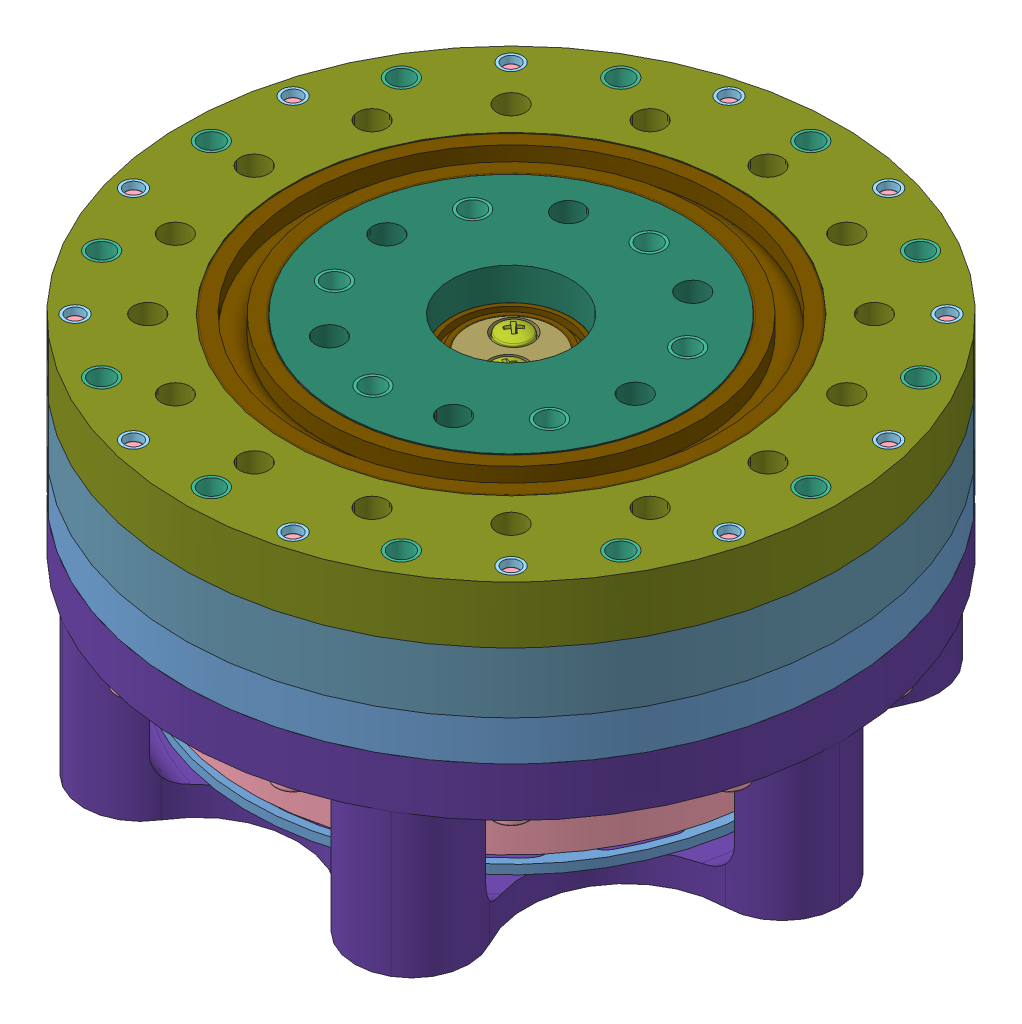
SolidWorks assembly Cycloidal, configuration Default. Lengths in mm. (continued)
Components (placement in the parent): (continued)
- foc-motor-controller.step-1: foc-motor-controller.step [Default] at (47.267 33.6573 89.1587) x (0.707107 0 0.707107) z (0 -1 0) size (57.23 50 8.13) (continued)
  - R_0603_1608Metric.step-6: R_0603_1608Metric.step [Default] at (10.9 4.1 1.595) size (1.6 0.8 0.45)
  - C_1206_3216Metric.step-2: C_1206_3216Metric.step [Default] at (6.3 11 1.595) x (0 1 0) z (0 0 1) size (3.2 1.6 1.6)
  - XT30PW_2_2_-M.G.B.step-1: XT30PW_2_2_-M.G.B.step [Default] at (-20.5 9.5 1.595) x (0 -1 0) z (-1 0 0) size (15.5 7.1 12.53)
  - R_0603_1608Metric.step-7: R_0603_1608Metric.step [Default] at (0.3 -11.1 1.595) size (1.6 0.8 0.45)
  - C_0603_1608Metric.step-6: C_0603_1608Metric.step [Default] at (19 -0.4 1.595) x (-0.707107 -0.707107 0) z (0 0 1) size (1.6 0.8 0.8)
  - C_1206_3216Metric.step-3: C_1206_3216Metric.step [Default] at (13.3 11 1.595) x (0 1 0) z (0 0 1) size (3.2 1.6 1.6)
  - R_0603_1608Metric.step-8: R_0603_1608Metric.step [Default] at (10.2 -7.375 1.595) x (0 -1 0) z (0 0 1) size (1.6 0.8 0.45)
  - JST_GH_SM08B-GHS-TB_1x08-1MP_P1.25mm_Horizontal.step-1: JST_GH_SM08B-GHS-TB_1x08-1MP_P1.25mm_Horizontal.step [Default] at (10 -22 1.595) size (13.25 4.95 4.25)
  - C_1206_3216Metric.step-4: C_1206_3216Metric.step [Default] at (-12.3 11 1.595) x (0 1 0) z (0 0 1) size (3.2 1.6 1.6)
  - JST_GH_SM06B-GHS-TB_1x06-1MP_P1.25mm_Horizontal.step-1: JST_GH_SM06B-GHS-TB_1x06-1MP_P1.25mm_Horizontal.step [Default] at (-4.3 -22 1.595) size (10.75 4.95 4.25)
  - C_0603_1608Metric.step-7: C_0603_1608Metric.step [Default] at (7.3 -4.5 1.595) x (-1 0 0) z (0 0 1) size (1.6 0.8 0.8)
  - R_0603_1608Metric.step-9: R_0603_1608Metric.step [Default] at (18.1 -3.86 1.595) x (-1 0 0) z (0 0 1) size (1.6 0.8 0.45)
  - C_1206_3216Metric.step-5: C_1206_3216Metric.step [Default] at (22.6794 -1.2206 1.595) x (0.707107 -0.707107 0) z (0 0 1) size (3.2 1.6 1.6)
  - R_Array_Convex_4x0402.step-1: R_Array_Convex_4x0402.step [Default] at (6.8 -2.5 1.595) size (1 2 0.35)
  - R_0603_1608Metric.step-10: R_0603_1608Metric.step [Default] at (7.7 -16.8 1.595) x (0 -1 0) z (0 0 1) size (1.6 0.8 0.45)
  - C_1206_3216Metric.step-6: C_1206_3216Metric.step [Default] at (8.7 11 1.595) x (0 1 0) z (0 0 1) size (3.2 1.6 1.6)
  - C_0603_1608Metric.step-8: C_0603_1608Metric.step [Default] at (16.1 -11.3 1.595) x (0 1 0) z (0 0 1) size (1.6 0.8 0.8)
  - SOT-23-5.step-1: SOT-23-5.step [Default] at (-3.1 -16.6 1.595) x (-1 0 0) z (0 0 1) size (2.8 2.9 1.55)
  - C_0603_1608Metric.step-9: C_0603_1608Metric.step [Default] at (17.8 -13.6 1.595) size (1.6 0.8 0.8)
  - R_0603_1608Metric.step-11: R_0603_1608Metric.step [Default] at (-11.5 -20.3875 1.595) x (0 -1 0) z (0 0 1) size (1.6 0.8 0.45)
  - C_0603_1608Metric.step-10: C_0603_1608Metric.step [Default] at (-12.4 2.3 1.595) x (0 1 0) z (0 0 1) size (1.6 0.8 0.8)
  - C_1206_3216Metric.step-7: C_1206_3216Metric.step [Default] at (18 11 1.595) x (0 1 0) z (0 0 1) size (3.2 1.6 1.6)
  - R_0603_1608Metric.step-12: R_0603_1608Metric.step [Default] at (-10.8105 -14.9971 1.595) x (-1 0 0) z (0 0 1) size (1.6 0.8 0.45)
  - C_0603_1608Metric.step-11: C_0603_1608Metric.step [Default] at (-13.8 -9.4 1.595) x (-1 0 0) z (0 0 1) size (1.6 0.8 0.8)
  - R_0603_1608Metric.step-13: R_0603_1608Metric.step [Default] at (-23.15 -14.5 1.595) x (-1 0 0) z (0 0 1) size (1.6 0.8 0.45)
  - C_0603_1608Metric.step-12: C_0603_1608Metric.step [Default] at (1.1 -0.2 1.595) x (0 1 0) z (0 0 1) size (1.6 0.8 0.8)
  - D_0805_2012Metric.step-1: D_0805_2012Metric.step [Default] at (22.9 -9.6 1.595) x (0 1 0) z (0 0 1) size (2 1.27 0.8)
  - C_0603_1608Metric.step-13: C_0603_1608Metric.step [Default] at (-7.8 3.775 1.595) x (0 -1 0) z (0 0 1) size (1.6 0.8 0.8)
  - R_0603_1608Metric.step-14: R_0603_1608Metric.step [Default] at (-6.4 -12.825 1.595) x (0 1 0) z (0 0 1) size (1.6 0.8 0.45)
  - L_0603_1608Metric.step-1: L_0603_1608Metric.step [Default] at (-10.1 3 1.595) size (1.6 0.8 0.8)
  - C_0603_1608Metric.step-14: C_0603_1608Metric.step [Default] at (17.9 0.7 1.595) x (-0.707107 -0.707107 0) z (0 0 1) size (1.6 0.8 0.8)
  - HVSSOP-10.step-1: HVSSOP-10.step [Default] at (18.6 -9.6 1.595) x (0 -1 0) z (-1 0 0) size (4.9 1.1 3)
  - C_0603_1608Metric.step-15: C_0603_1608Metric.step [Default] at (7.9 4.1 1.595) x (-1 0 0) z (0 0 1) size (1.6 0.8 0.8)
  - C_0603_1608Metric.step-16: C_0603_1608Metric.step [Default] at (21.1 -9.6 1.595) x (0 -1 0) z (0 0 1) size (1.6 0.8 0.8)
  - R_0603_1608Metric.step-15: R_0603_1608Metric.step [Default] at (-10.8105 -11.9971 1.595) x (-1 0 0) z (0 0 1) size (1.6 0.8 0.45)
  - R_0603_1608Metric.step-16: R_0603_1608Metric.step [Default] at (-18.2 -17.4 1.595) size (1.6 0.8 0.45)
  - C_1206_3216Metric.step-8: C_1206_3216Metric.step [Default] at (-3 11 1.595) x (0 1 0) z (0 0 1) size (3.2 1.6 1.6)
  - R_0603_1608Metric.step-17: R_0603_1608Metric.step [Default] at (-16.9 -20.4 1.595) x (0 -1 0) z (0 0 1) size (1.6 0.8 0.45)
  - R_0603_1608Metric.step-18: R_0603_1608Metric.step [Default] at (-13.3 -20.3875 1.595) x (0 -1 0) z (0 0 1) size (1.6 0.8 0.45)
  - R_0603_1608Metric.step-19: R_0603_1608Metric.step [Default] at (-15.1 -20.3875 1.595) x (0 -1 0) z (0 0 1) size (1.6 0.8 0.45)
  - C_0603_1608Metric.step-17: C_0603_1608Metric.step [Default] at (15.5 -14.4 1.595) x (0 -1 0) z (0 0 1) size (1.6 0.8 0.8)
  - LED_0603_1608Metric.step-1: LED_0603_1608Metric.step [Default] at (-11.5 -23.3875 1.595) x (0 1 0) z (0 0 1) size (1.6 0.8 1.1)
  - C_0805_2012Metric.step-1: C_0805_2012Metric.step [Default] at (19.95 -17 1.595) size (2 1.25 1.25)
  - D_SMB.step-1: D_SMB.step [Default] at (-16.5 11.208 1.595) x (0 -1 0) z (0 0 1) size (5.3 3.55 2.15)
  - C_1206_3216Metric.step-9: C_1206_3216Metric.step [Default] at (-5.3 11 1.595) x (0 1 0) z (0 0 1) size (3.2 1.6 1.6)
  - XT30PW_2_2_-M.G.B.step-2: XT30PW_2_2_-M.G.B.step [Default] at (-20.5 -6.5 1.595) x (0 -1 0) z (-1 0 0) size (15.5 7.1 12.53)
  - C_1206_3216Metric.step-10: C_1206_3216Metric.step [Default] at (1.7 11 1.595) x (0 1 0) z (0 0 1) size (3.2 1.6 1.6)
  - C_1206_3216Metric.step-11: C_1206_3216Metric.step [Default] at (11 11 1.595) x (0 1 0) z (0 0 1) size (3.2 1.6 1.6)
  - C_0603_1608Metric.step-18: C_0603_1608Metric.step [Default] at (-6.3 3.775 1.595) x (0 -1 0) z (0 0 1) size (1.6 0.8 0.8)
  - C_0603_1608Metric.step-19: C_0603_1608Metric.step [Default] at (16.8686 1.7314 1.595) x (0.707107 0.707107 0) z (0 0 1) size (1.6 0.8 0.8)
  - C_0603_1608Metric.step-20: C_0603_1608Metric.step [Default] at (-15.0105 -11.1 1.595) size (1.6 0.8 0.8)
  - C_1206_3216Metric.step-12: C_1206_3216Metric.step [Default] at (-7.7 11 1.595) x (0 1 0) z (0 0 1) size (3.2 1.6 1.6)
  - C_0603_1608Metric.step-21: C_0603_1608Metric.step [Default] at (-18.2 -15.8 1.595) size (1.6 0.8 0.8)
  - C_0603_1608Metric.step-22: C_0603_1608Metric.step [Default] at (-2.1 -11.3 1.595) x (0 -1 0) z (0 0 1) size (1.6 0.8 0.8)
  - C_0603_1608Metric.step-23: C_0603_1608Metric.step [Default] at (-10.8105 -13.4971 1.595) size (1.6 0.8 0.8)
  - C_1206_3216Metric.step-13: C_1206_3216Metric.step [Default] at (4 11 1.595) x (0 1 0) z (0 0 1) size (3.2 1.6 1.6)
  - R_0603_1608Metric.step-20: R_0603_1608Metric.step [Default] at (16 -17.8 1.595) x (0 1 0) z (0 0 1) size (1.6 0.8 0.45)
  - Texas_S-PVSON-N8.step-1: Texas_S-PVSON-N8.step [Default] at (-14.4105 -13.7 1.595) x (-1 0 0) z (0 0 1) size (3 2.98 0.92)
  - C_1206_3216Metric.step-14: C_1206_3216Metric.step [Default] at (21 -2.9 1.595) x (0.707107 -0.707107 0) z (0 0 1) size (3.2 1.6 1.6)
  - C_0603_1608Metric.step-24: C_0603_1608Metric.step [Default] at (-5.9 -16.6 1.595) x (0 1 0) z (0 0 1) size (1.6 0.8 0.8)
  - C_0603_1608Metric.step-25: C_0603_1608Metric.step [Default] at (-3.1 -14.1 1.595) size (1.6 0.8 0.8)
  - R_0603_1608Metric.step-21: R_0603_1608Metric.step [Default] at (7.2 -7.375 1.595) x (0 -1 0) z (0 0 1) size (1.6 0.8 0.45)
  - C_1206_3216Metric.step-15: C_1206_3216Metric.step [Default] at (-0.7 11 1.595) x (0 1 0) z (0 0 1) size (3.2 1.6 1.6)
  - LQFP-64_10x10mm_P0.5mm.step-1: LQFP-64_10x10mm_P0.5mm.step [Default] at (-7 -4.5 1.595) x (-1 0 0) z (0 0 1) size (12 12 1.5)
  - C_0805_2012Metric.step-2: C_0805_2012Metric.step [Default] at (23.35 -17 1.595) x (-1 0 0) z (0 0 1) size (2 1.25 1.25)
  - C_0603_1608Metric.step-26: C_0603_1608Metric.step [Default] at (10.8 -16.8 1.595) x (0 -1 0) z (0 0 1) size (1.6 0.8 0.8)
  - R_0603_1608Metric.step-22: R_0603_1608Metric.step [Default] at (17.5 -17.8 1.595) x (0 -1 0) z (0 0 1) size (1.6 0.8 0.45)
  - C_1206_3216Metric.step-16: C_1206_3216Metric.step [Default] at (20.3 11 1.595) x (0 1 0) z (0 0 1) size (3.2 1.6 1.6)
  - R_0603_1608Metric.step-23: R_0603_1608Metric.step [Default] at (9.2 -16.8 1.595) x (0 -1 0) z (0 0 1) size (1.6 0.8 0.45)
  - C_1206_3216Metric.step-17: C_1206_3216Metric.step [Default] at (-10 11 1.595) x (0 1 0) z (0 0 1) size (3.2 1.6 1.6)
  - R_0603_1608Metric.step-24: R_0603_1608Metric.step [Default] at (17.8 -15.2 1.595) size (1.6 0.8 0.45)
  - C_1206_3216Metric.step-18: C_1206_3216Metric.step [Default] at (19.9 2.6 1.595) x (-0.707107 0.707107 0) z (0 0 1) size (3.2 1.6 1.6)
  - C_0603_1608Metric.step-27: C_0603_1608Metric.step [Default] at (13.4 -7.375 1.595) x (0 -1 0) z (0 0 1) size (1.6 0.8 0.8)
  - R_0603_1608Metric.step-25: R_0603_1608Metric.step [Default] at (8.7 -7.375 1.595) x (0 -1 0) z (0 0 1) size (1.6 0.8 0.45)
  - PQFN-8-EP_6x5mm_P1.27mm_Generic.step-1: PQFN-8-EP_6x5mm_P1.27mm_Generic.step [Default] at (4.9 14.4 -0.085) x (0 1 0) z (0 0 -1) size (6.15 5.15 1.09)
  - C_0805_2012Metric.step-3: C_0805_2012Metric.step [Default] at (-3 8.9 -0.085) x (0 1 0) z (0 0 -1) size (2 1.25 1.25)
  - C_0603_1608Metric.step-28: C_0603_1608Metric.step [Default] at (1.5 -4.3 -0.085) x (0 1 0) z (0 0 -1) size (1.6 0.8 0.8)
  - R_2512_6332Metric.step-1: R_2512_6332Metric.step [Default] at (2.1 8.6 -0.085) x (-1 0 0) z (0 0 -1) size (6.3 3.2 0.6)
  - C_0805_2012Metric.step-4: C_0805_2012Metric.step [Default] at (18.8 8.9 -0.085) x (0 1 0) z (0 0 -1) size (2 1.25 1.25)
  - C_0805_2012Metric.step-5: C_0805_2012Metric.step [Default] at (-5.2 8.901 -0.085) x (0 1 0) z (0 0 -1) size (2 1.25 1.25)
  - PQFN-8-EP_6x5mm_P1.27mm_Generic.step-2: PQFN-8-EP_6x5mm_P1.27mm_Generic.step [Default] at (16.9 14.6 -0.085) x (0 -1 0) z (0 0 -1) size (6.15 5.15 1.09)
  - PQFN-8-EP_6x5mm_P1.27mm_Generic.step-3: PQFN-8-EP_6x5mm_P1.27mm_Generic.step [Default] at (-1.1 14.6 -0.085) x (0 -1 0) z (0 0 -1) size (6.15 5.15 1.09)
  - R_0603_1608Metric.step-26: R_0603_1608Metric.step [Default] at (8.2 8.8 -0.085) x (0 1 0) z (0 0 -1) size (1.6 0.8 0.45)
  - R_2512_6332Metric.step-2: R_2512_6332Metric.step [Default] at (-10.3 8.601 -0.085) x (1 0 0) z (0 0 -1) size (6.3 3.2 0.6)
  - TSSOP-16_4.4x5mm_P0.65mm.step-1: TSSOP-16_4.4x5mm_P0.65mm.step [Default] at (0 0 -0.085) x (-1 0 0) z (0 0 -1) size (6.4 5 1.1)
  - C_0603_1608Metric.step-29: C_0603_1608Metric.step [Default] at (0 -4.25 -0.085) x (0 1 0) z (0 0 -1) size (1.6 0.8 0.8)
  - PQFN-8-EP_6x5mm_P1.27mm_Generic.step-4: PQFN-8-EP_6x5mm_P1.27mm_Generic.step [Default] at (10.9 14.4 -0.085) x (0 1 0) z (0 0 -1) size (6.15 5.15 1.09)
  - R_2512_6332Metric.step-3: R_2512_6332Metric.step [Default] at (13.7 8.6 -0.085) x (1 0 0) z (0 0 -1) size (6.3 3.2 0.6)
  - PQFN-8-EP_6x5mm_P1.27mm_Generic.step-5: PQFN-8-EP_6x5mm_P1.27mm_Generic.step [Default] at (-13.1 14.401 -0.085) x (0 1 0) z (0 0 -1) size (6.15 5.15 1.09)
  - C_0603_1608Metric.step-30: C_0603_1608Metric.step [Default] at (-1.5 -4.3 -0.085) x (0 -1 0) z (0 0 -1) size (1.6 0.8 0.8)
  - PQFN-8-EP_6x5mm_P1.27mm_Generic.step-6: PQFN-8-EP_6x5mm_P1.27mm_Generic.step [Default] at (-7.1 14.601 -0.085) x (0 -1 0) z (0 0 -1) size (6.15 5.15 1.09)
  - foc-motor-controller_PCB.step-1: foc-motor-controller_PCB.step [Default] at origin size (50 50 1.51)
- hex nut style 1 gradeab_iso-1: hex nut style 1 gradeab_iso [ISO - 4032 - M3 - W - N] at (47.267 33.6573 58.7531) x (1 0 0) z (0 -1 0) size (5.5 6.35 2.4)
Mates (geometry in assembly coordinates):
- Coincident1: coincident anti-aligned: plane of motor-X83008S.stp-1/outrunner.stp-1 through (20.8832 69.6573 111.3881) normal (0 1 0); plane of Base_Plate-1 through (47.267 69.6573 89.1587) normal (0 -1 0)
- Concentric1: concentric anti-aligned: line of motor-X83008S.stp-1/outrunner.stp-1 through (35.4134 64.1573 99.1458) axis (0 1 0); cylinder of Base_Plate-1 through (35.4134 76.6573 99.1458) axis (0 -1 0) radius 1.5
- Concentric2: concentric anti-aligned: cylinder of motor-X83008S.stp-1/shaft.stp-1 through (47.267 69.6573 89.1587) axis (0 1 0) radius 1.5; line of Base_Plate-1 through (47.267 76.6573 89.1587) axis (0 -1 0)
- Coincident2: coincident anti-aligned: plane of Base_Plate-1 through (47.267 76.6573 89.1587) normal (0 1 0); plane of Eccentric_Shaft-1/Eccentric_Shaft_bot-1 through (48.4141 76.6573 88.1922) normal (0 -1 0)
- Concentric75: concentric anti-aligned: cylinder of Output_Shaft-1 through (47.267 97.2573 89.1587) axis (0 -1 0) radius 30; cylinder of radial ball bearing_68_iso-39 through (47.267 71.6198 89.1587) axis (0 1 0) radius 30
- Concentric76: concentric anti-aligned: cylinder of Cover-1 through (47.267 97.2573 89.1587) axis (0 -1 0) radius 39; cylinder of radial ball bearing_68_iso-39 through (47.267 71.6198 89.1587) axis (0 1 0) radius 39
- Coincident104: coincident aligned: plane of Cover-1 through (47.267 97.2573 89.1587) normal (0 1 0); plane of radial ball bearing_68_iso-39 through (8.567 97.2573 89.1587) normal (0 1 0)
- Coincident105: coincident aligned: plane of Output_Shaft-1 through (47.267 97.2573 89.1587) normal (0 1 0); plane of Cover-1 through (47.267 97.2573 89.1587) normal (0 1 0)
- Concentric77: concentric aligned: cylinder of Ring_Pin_Housing-1 through (47.267 87.2573 89.1587) axis (0 -1 0) radius 57.5; cylinder of Motor_Cover-2 through (47.267 69.6573 89.1587) axis (0 -1 0) radius 57.5
- Concentric78: concentric anti-aligned: cylinder of Base_Plate-1 through (47.267 76.6573 89.1587) axis (0 -1 0) radius 20; cylinder of radial ball bearing_68_iso-40 through (47.267 52.3198 89.1587) axis (0 1 0) radius 20
- Concentric79: concentric aligned: cylinder of Ring_Pin_Housing-1 through (9.0832 87.2573 50.9749) axis (0 -1 0) radius 1.6; cylinder of Base_plate_2-1 through (9.0832 76.6573 50.9749) axis (0 -1 0) radius 1.75
- Concentric80: concentric aligned: cylinder of Ring_Pin_Housing-1 through (47.267 87.2573 89.1587) axis (0 -1 0) radius 57.5; cylinder of Base_plate_2-1 through (47.267 76.6573 89.1587) axis (0 -1 0) radius 57.5
- Coincident107: coincident anti-aligned: plane of Ring_Pin_Housing-1 through (47.267 76.6573 89.1587) normal (0 -1 0); plane of Base_plate_2-1 through (47.267 76.6573 89.1587) normal (0 1 0)
- Concentric83: concentric aligned: cylinder of Ring_Pin_Housing-1 through (9.0832 87.2573 50.9749) axis (0 -1 0) radius 1.6; cylinder of Cover-1 through (9.0832 97.2573 50.9749) axis (0 -1 0) radius 2
- Concentric84: concentric aligned: cylinder of Cover-1 through (15.4472 87.2573 57.3389) axis (0 1 0) radius 2.5; cylinder of m13_bearing-1/m6-1 through (15.4472 86.8573 57.3389) axis (0 1 0) radius 2
- Concentric85: concentric aligned: cylinder of Cover-1 through (47.267 87.2573 134.1587) axis (0 1 0) radius 2.5; cylinder of m13_bearing-11/m6-1 through (47.267 86.8573 134.1587) axis (0 1 0) radius 2
- Concentric86: concentric aligned: cylinder of Cover-1 through (64.4877 87.2573 130.7332) axis (0 1 0) radius 2.5; cylinder of m13_bearing-2/m6-1 through (64.4877 86.8573 130.7332) axis (0 1 0) radius 2
- Concentric87: concentric aligned: cylinder of Cover-1 through (79.0868 87.2573 120.9785) axis (0 1 0) radius 2.5; cylinder of m13_bearing-12/m6-1 through (79.0868 86.8573 120.9785) axis (0 1 0) radius 2
- Concentric88: concentric aligned: cylinder of Cover-1 through (88.8416 87.2573 106.3794) axis (0 1 0) radius 2.5; cylinder of m13_bearing-5/m6-1 through (88.8416 86.8573 106.3794) axis (0 1 0) radius 2
- Concentric89: concentric aligned: cylinder of Cover-1 through (92.267 87.2573 89.1587) axis (0 1 0) radius 2.5; cylinder of m13_bearing-4/m6-1 through (92.267 86.8573 89.1587) axis (0 1 0) radius 2
- Concentric90: concentric aligned: cylinder of Cover-1 through (30.0462 87.2573 47.5841) axis (0 1 0) radius 2.5; cylinder of m13_bearing-6/m6-1 through (30.0462 86.8573 47.5841) axis (0 1 0) radius 2
- Concentric91: concentric aligned: cylinder of Cover-1 through (47.267 87.2573 44.1587) axis (0 1 0) radius 2.5; cylinder of m13_bearing-3/m6-1 through (47.267 86.8573 44.1587) axis (0 1 0) radius 2
- Concentric92: concentric aligned: cylinder of Cover-1 through (64.4877 87.2573 47.5841) axis (0 1 0) radius 2.5; cylinder of m13_bearing-7/m6-1 through (64.4877 86.8573 47.5841) axis (0 1 0) radius 2
- Concentric93: concentric aligned: cylinder of Cover-1 through (79.0868 87.2573 57.3389) axis (0 1 0) radius 2.5; cylinder of m13_bearing-8/m6-1 through (79.0868 86.8573 57.3389) axis (0 1 0) radius 2
- Concentric94: concentric aligned: cylinder of Cover-1 through (88.8416 87.2573 71.9379) axis (0 1 0) radius 2.5; cylinder of m13_bearing-9/m6-1 through (88.8416 86.8573 71.9379) axis (0 1 0) radius 2
- Concentric96: concentric aligned: cylinder of Base_plate_2-1 through (47.267 76.6573 134.1587) axis (0 -1 0) radius 2.5; cylinder of socket button head screw_iso-2 through (47.267 67.4573 134.1587) axis (0 -1 0) radius 2
- Coincident121: coincident anti-aligned: plane of Base_plate_2-1 through (47.267 69.6573 89.1587) normal (0 -1 0); plane of socket button head screw_iso-2 through (45.8877 69.6573 132.7104) normal (0 1 0)
- Concentric971: concentric aligned: cylinder of Base_plate_2-1 through (15.4472 76.6573 57.3389) axis (0 -1 0) radius 2.5; cylinder of socket button head screw_iso-3 through (15.4472 67.4573 57.3389) axis (0 -1 0) radius 3.8
- Coincident1221: coincident anti-aligned: plane of Base_plate_2-1 through (47.267 69.6573 89.1587) normal (0 -1 0); plane of socket button head screw_iso-3 through (14.0679 69.6573 55.8906) normal (0 1 0)
- Concentric981: concentric aligned: cylinder of Base_plate_2-1 through (30.0462 76.6573 47.5841) axis (0 -1 0) radius 2.5; cylinder of socket button head screw_iso-4 through (30.0462 67.4573 47.5841) axis (0 -1 0) radius 3.8
- Coincident1231: coincident anti-aligned: plane of Base_plate_2-1 through (47.267 69.6573 89.1587) normal (0 -1 0); plane of socket button head screw_iso-4 through (28.6669 69.6573 46.1358) normal (0 1 0)
- Concentric991: concentric aligned: cylinder of Base_plate_2-1 through (47.267 76.6573 44.1587) axis (0 -1 0) radius 2.5; cylinder of socket button head screw_iso-5 through (47.267 67.4573 44.1587) axis (0 -1 0) radius 3.8
- Coincident1241: coincident anti-aligned: plane of Base_plate_2-1 through (47.267 69.6573 89.1587) normal (0 -1 0); plane of socket button head screw_iso-5 through (45.8877 69.6573 42.7104) normal (0 1 0)
- Concentric1001: concentric aligned: cylinder of Base_plate_2-1 through (64.4877 76.6573 47.5841) axis (0 -1 0) radius 2.5; cylinder of socket button head screw_iso-6 through (64.4877 67.4573 47.5841) axis (0 -1 0) radius 3.8
- Coincident1251: coincident anti-aligned: plane of Base_plate_2-1 through (47.267 69.6573 89.1587) normal (0 -1 0); plane of socket button head screw_iso-6 through (63.1085 69.6573 46.1358) normal (0 1 0)
- Concentric1021: concentric aligned: cylinder of Base_plate_2-1 through (88.8416 76.6573 71.9379) axis (0 -1 0) radius 2.5; cylinder of socket button head screw_iso-8 through (88.8416 67.4573 71.9379) axis (0 -1 0) radius 3.8
- Coincident1271: coincident anti-aligned: plane of Base_plate_2-1 through (47.267 69.6573 89.1587) normal (0 -1 0); plane of socket button head screw_iso-8 through (87.4623 69.6573 70.4896) normal (0 1 0)
- Concentric1031: concentric aligned: cylinder of Base_plate_2-1 through (92.267 76.6573 89.1587) axis (0 -1 0) radius 2.5; cylinder of socket button head screw_iso-9 through (92.267 67.4573 89.1587) axis (0 -1 0) radius 3.8
- Coincident1281: coincident anti-aligned: plane of Base_plate_2-1 through (47.267 69.6573 89.1587) normal (0 -1 0); plane of socket button head screw_iso-9 through (90.8877 69.6573 87.7104) normal (0 1 0)
- Concentric1041: concentric aligned: cylinder of Base_plate_2-1 through (88.8416 76.6573 106.3794) axis (0 -1 0) radius 2.5; cylinder of socket button head screw_iso-10 through (88.8416 67.4573 106.3794) axis (0 -1 0) radius 3.8
- Coincident1291: coincident anti-aligned: plane of Base_plate_2-1 through (47.267 69.6573 89.1587) normal (0 -1 0); plane of socket button head screw_iso-10 through (87.4623 69.6573 104.9311) normal (0 1 0)
- Concentric1051: concentric aligned: cylinder of Base_plate_2-1 through (79.0868 76.6573 120.9785) axis (0 -1 0) radius 2.5; cylinder of socket button head screw_iso-11 through (79.0868 67.4573 120.9785) axis (0 -1 0) radius 3.8
- Coincident1301: coincident anti-aligned: plane of Base_plate_2-1 through (47.267 69.6573 89.1587) normal (0 -1 0); plane of socket button head screw_iso-11 through (77.7075 69.6573 119.5302) normal (0 1 0)
- Coincident132: coincident anti-aligned: plane of Ring_Pin_Housing-1 through (47.267 87.2573 89.1587) normal (0 1 0); plane of Cover-1 through (47.267 87.2573 89.1587) normal (0 -1 0)
- Coincident133: coincident anti-aligned: plane of Motor_Cover-2 through (47.267 69.6573 89.1587) normal (0 1 0); plane of Base_plate_2-1 through (47.267 69.6573 89.1587) normal (0 -1 0)
- Concentric109: concentric anti-aligned: cylinder of Output_Shaft-1 through (24.2995 97.2573 87.9364) axis (0 -1 0) radius 2.5; cylinder of m13_bearing-14/m6-1 through (24.2995 86.4573 87.9364) axis (0 1 0) radius 2
- Concentric110: concentric anti-aligned: cylinder of Output_Shaft-1 through (36.8417 97.2573 68.6571) axis (0 -1 0) radius 2.5; cylinder of m13_bearing-13/m6-1 through (36.8417 86.4573 68.6571) axis (0 1 0) radius 2
- Concentric111: concentric anti-aligned: cylinder of Output_Shaft-1 through (59.8092 97.2573 69.8794) axis (0 -1 0) radius 2.5; cylinder of m13_bearing-16/m6-1 through (59.8092 86.4573 69.8794) axis (0 1 0) radius 2
- Concentric112: concentric anti-aligned: cylinder of Output_Shaft-1 through (70.2345 97.2573 90.3809) axis (0 -1 0) radius 2.5; cylinder of m13_bearing-18/m6-1 through (70.2345 86.4573 90.3809) axis (0 1 0) radius 2
- Concentric113: concentric anti-aligned: cylinder of Output_Shaft-1 through (57.6922 97.2573 109.6602) axis (0 -1 0) radius 2.5; cylinder of m13_bearing-17/m6-1 through (57.6922 86.4573 109.6602) axis (0 1 0) radius 2
- Concentric114: concentric anti-aligned: cylinder of Output_Shaft-1 through (34.7247 97.2573 108.438) axis (0 -1 0) radius 2.5; cylinder of m13_bearing-15/m6-1 through (34.7247 86.4573 108.438) axis (0 1 0) radius 2
- Coincident136: coincident aligned: plane of m13_bearing-13/m6-1 through (36.8417 92.4573 68.6571) normal (0 1 0); plane of m13_bearing-14/m6-1 through (24.2995 92.4573 87.9364) normal (0 1 0)
- Coincident137: coincident aligned: plane of m13_bearing-14/m6-1 through (24.2995 92.4573 87.9364) normal (0 1 0); plane of m13_bearing-16/m6-1 through (59.8092 92.4573 69.8794) normal (0 1 0)
- Coincident138: coincident aligned: plane of m13_bearing-14/m6-1 through (24.2995 92.4573 87.9364) normal (0 1 0); plane of m13_bearing-18/m6-1 through (70.2345 92.4573 90.3809) normal (0 1 0)
- Coincident139: coincident aligned: plane of m13_bearing-14/m6-1 through (24.2995 92.4573 87.9364) normal (0 1 0); plane of m13_bearing-17/m6-1 through (57.6922 92.4573 109.6602) normal (0 1 0)
- Coincident140: coincident aligned: plane of m13_bearing-14/m6-1 through (24.2995 92.4573 87.9364) normal (0 1 0); plane of m13_bearing-15/m6-1 through (34.7247 92.4573 108.438) normal (0 1 0)
- Concentric117: concentric anti-aligned: cylinder of Cover-1 through (9.0832 97.2573 127.3424) axis (0 -1 0) radius 2; cylinder of Motor_Cover-2 through (9.0832 59.6573 127.3424) axis (0 1 0) radius 1.75
- Concentric118: concentric anti-aligned: cylinder of Output_Shaft-1 through (36.8417 97.2573 68.6571) axis (0 -1 0) radius 2.5; cylinder of M4x6x5.5_brass_insert-1 through (36.8417 86.4573 68.6571) axis (0 1 0) radius 2
- Coincident144: coincident aligned: plane of Cover-1 through (47.267 97.2573 89.1587) normal (0 1 0); plane of M3x4x4.2_brass_insert-1 through (-2.9238 97.2573 74.8329) normal (0 1 0)
- Concentric1211: concentric aligned: cylinder of Cover-1 through (9.0832 97.2573 50.9749) axis (0 -1 0) radius 2; cylinder of M3x4x4.2_brass_insert-2 through (9.0832 92.3553 50.9749) axis (0 -1 0) radius 1.5
- Concentric1221: concentric aligned: cylinder of Cover-1 through (33.2908 97.2573 36.9987) axis (0 -1 0) radius 2; cylinder of M3x4x4.2_brass_insert-3 through (33.2908 92.3553 36.9987) axis (0 -1 0) radius 1.5
- Concentric1251: concentric aligned: cylinder of Cover-1 through (99.427 97.2573 75.1824) axis (0 -1 0) radius 2; cylinder of M3x4x4.2_brass_insert-6 through (99.427 92.3553 75.1824) axis (0 -1 0) radius 1.8
- Concentric1271: concentric anti-aligned: cylinder of Cover-1 through (85.4508 97.2573 127.3424) axis (0 -1 0) radius 2; cylinder of M3x4x4.2_brass_insert-8 through (85.4508 98.1594 127.3424) axis (0 1 0) radius 1.8
- Concentric1331: concentric aligned: cylinder of Cover-1 through (61.2432 97.2573 36.9987) axis (0 -1 0) radius 2; cylinder of M3x4x4.2_brass_insert-14 through (61.2432 92.3553 36.9987) axis (0 -1 0) radius 1.8
- Concentric1341: concentric anti-aligned: cylinder of Cover-1 through (85.4508 97.2573 50.9749) axis (0 -1 0) radius 2; cylinder of M3x4x4.2_brass_insert-15 through (85.4508 98.1594 50.9749) axis (0 1 0) radius 2
- Concentric1351: concentric aligned: cylinder of Cover-1 through (99.427 97.2573 103.1349) axis (0 -1 0) radius 2; cylinder of M3x4x4.2_brass_insert-16 through (99.427 92.3553 103.1349) axis (0 -1 0) radius 2
- Concentric1361: concentric aligned: cylinder of Cover-1 through (61.2432 97.2573 141.3187) axis (0 -1 0) radius 2; cylinder of M3x4x4.2_brass_insert-17 through (61.2432 92.3553 141.3187) axis (0 -1 0) radius 2
- Concentric1381: concentric aligned: cylinder of Cover-1 through (33.2908 97.2573 141.3187) axis (0 -1 0) radius 2; cylinder of M3x4x4.2_brass_insert-19 through (33.2908 92.3553 141.3187) axis (0 -1 0) radius 2
- Concentric1391: concentric aligned: cylinder of Cover-1 through (9.0832 97.2573 127.3424) axis (0 -1 0) radius 2; cylinder of M3x4x4.2_brass_insert-20 through (9.0832 92.3553 127.3424) axis (0 -1 0) radius 1.5
- Concentric1401: concentric aligned: cylinder of Cover-1 through (-4.893 97.2573 103.1349) axis (0 -1 0) radius 2; cylinder of M3x4x4.2_brass_insert-21 through (-4.893 92.3553 103.1349) axis (0 -1 0) radius 1.5
- Coincident205: coincident aligned: plane of M3x4x4.2_brass_insert-1 through (-2.9238 97.2573 74.8329) normal (0 1 0); plane of M3x4x4.2_brass_insert-2 through (8.0628 97.2573 49.8755) normal (0 1 0)
- Coincident206: coincident aligned: plane of M3x4x4.2_brass_insert-1 through (-2.9238 97.2573 74.8329) normal (0 1 0); plane of M3x4x4.2_brass_insert-3 through (32.5264 97.2573 35.708) normal (0 1 0)
- Coincident207: coincident aligned: plane of M3x4x4.2_brass_insert-1 through (-2.9238 97.2573 74.8329) normal (0 1 0); plane of M3x4x4.2_brass_insert-14 through (62.0075 97.2573 38.2893) normal (0 1 0)
- Coincident208: coincident aligned: plane of M3x4x4.2_brass_insert-1 through (-2.9238 97.2573 74.8329) normal (0 1 0); plane of M3x4x4.2_brass_insert-15 through (87.2451 97.2573 50.0916) normal (0 1 0)
- Coincident209: coincident aligned: plane of M3x4x4.2_brass_insert-1 through (-2.9238 97.2573 74.8329) normal (0 1 0); plane of M3x4x4.2_brass_insert-6 through (98.4066 97.2573 74.083) normal (0 1 0)
- Coincident210: coincident aligned: plane of M3x4x4.2_brass_insert-1 through (-2.9238 97.2573 74.8329) normal (0 1 0); plane of M3x4x4.2_brass_insert-16 through (98.4066 97.2573 102.0355) normal (0 1 0)
- Coincident211: coincident aligned: plane of M3x4x4.2_brass_insert-1 through (-2.9238 97.2573 74.8329) normal (0 1 0); plane of M3x4x4.2_brass_insert-8 through (83.51 97.2573 127.8255) normal (0 1 0)
- Coincident212: coincident aligned: plane of M3x4x4.2_brass_insert-1 through (-2.9238 97.2573 74.8329) normal (0 1 0); plane of M3x4x4.2_brass_insert-17 through (62.2636 97.2573 142.4181) normal (0 1 0)
- Coincident213: coincident aligned: plane of M3x4x4.2_brass_insert-1 through (-2.9238 97.2573 74.8329) normal (0 1 0); plane of M3x4x4.2_brass_insert-19 through (34.3112 97.2573 142.4181) normal (0 1 0)
- Coincident214: coincident aligned: plane of M3x4x4.2_brass_insert-1 through (-2.9238 97.2573 74.8329) normal (0 1 0); plane of M3x4x4.2_brass_insert-20 through (10.1036 97.2573 128.4419) normal (0 1 0)
- Coincident215: coincident aligned: plane of M3x4x4.2_brass_insert-1 through (-2.9238 97.2573 74.8329) normal (0 1 0); plane of M3x4x4.2_brass_insert-21 through (-3.8726 97.2573 104.2343) normal (0 1 0)
- Coincident1432: coincident aligned: plane of m13_bearing-13/m6-1 through (36.8417 92.4573 68.6571) normal (0 1 0); plane of M4x6x5.5_brass_insert-1 through (34.9772 92.4573 70.3224) normal (0 1 0)
- Concentric14021: concentric aligned: cylinder of Output_Shaft-1 through (70.2345 97.2573 90.3809) axis (0 -1 0) radius 2.5; cylinder of M4x6x5.5_brass_insert-4 through (70.2345 80.5133 90.3809) axis (0 -1 0) radius 2.5
- Concentric14031: concentric aligned: cylinder of Output_Shaft-1 through (57.6922 97.2573 109.6602) axis (0 -1 0) radius 2.5; cylinder of M4x6x5.5_brass_insert-5 through (57.6922 80.5133 109.6602) axis (0 -1 0) radius 2.5
- Concentric14041: concentric aligned: cylinder of Output_Shaft-1 through (34.7247 97.2573 108.438) axis (0 -1 0) radius 2.5; cylinder of M4x6x5.5_brass_insert-6 through (34.7247 80.5133 108.438) axis (0 -1 0) radius 2.5
- Concentric14051: concentric aligned: cylinder of Output_Shaft-1 through (24.2995 97.2573 87.9364) axis (0 -1 0) radius 2.5; cylinder of M4x6x5.5_brass_insert-7 through (24.2995 80.5133 87.9364) axis (0 -1 0) radius 2.5
- Concentric14061: concentric aligned: cylinder of Output_Shaft-1 through (48.4892 97.2573 66.1912) axis (0 -1 0) radius 2.5; cylinder of M4x6x5.5_brass_insert-8 through (48.4892 85.3133 66.1912) axis (0 -1 0) radius 2.5
- Concentric14071: concentric aligned: cylinder of Output_Shaft-1 through (27.9877 97.2573 76.6164) axis (0 -1 0) radius 2.5; cylinder of M4x6x5.5_brass_insert-9 through (27.9877 85.3133 76.6164) axis (0 -1 0) radius 2.5
- Concentric14081: concentric aligned: cylinder of Output_Shaft-1 through (26.7654 97.2573 99.5839) axis (0 -1 0) radius 2.5; cylinder of M4x6x5.5_brass_insert-10 through (26.7654 85.3133 99.5839) axis (0 -1 0) radius 2.5
- Concentric14091: concentric aligned: cylinder of Output_Shaft-1 through (46.0447 97.2573 112.1262) axis (0 -1 0) radius 2.5; cylinder of M4x6x5.5_brass_insert-11 through (46.0447 85.3133 112.1262) axis (0 -1 0) radius 2.5
- Concentric14111: concentric aligned: cylinder of Output_Shaft-1 through (66.5463 97.2573 101.7009) axis (0 -1 0) radius 2.5; cylinder of M4x6x5.5_brass_insert-13 through (66.5463 85.3133 101.7009) axis (0 -1 0) radius 2.5
- Concentric14121: concentric aligned: cylinder of Output_Shaft-1 through (67.7686 97.2573 78.7334) axis (0 -1 0) radius 2.5; cylinder of M4x6x5.5_brass_insert-14 through (67.7686 85.3133 78.7334) axis (0 -1 0) radius 2.5
- Concentric14131: concentric aligned: cylinder of Output_Shaft-1 through (59.8092 97.2573 69.8794) axis (0 -1 0) radius 2.5; cylinder of M4x6x5.5_brass_insert-15 through (59.8092 80.5133 69.8794) axis (0 -1 0) radius 2.5
- Coincident1435: coincident aligned: plane of M4x6x5.5_brass_insert-1 through (34.9772 92.4573 70.3224) normal (0 1 0); plane of M4x6x5.5_brass_insert-15 through (59.8092 92.4573 69.8794) normal (0 1 0)
- Coincident1436: coincident aligned: plane of M4x6x5.5_brass_insert-1 through (34.9772 92.4573 70.3224) normal (0 1 0); plane of M4x6x5.5_brass_insert-4 through (70.2345 92.4573 90.3809) normal (0 1 0)
- Coincident1437: coincident aligned: plane of M4x6x5.5_brass_insert-1 through (34.9772 92.4573 70.3224) normal (0 1 0); plane of M4x6x5.5_brass_insert-5 through (57.6922 92.4573 109.6602) normal (0 1 0)
- Coincident1438: coincident aligned: plane of M4x6x5.5_brass_insert-1 through (34.9772 92.4573 70.3224) normal (0 1 0); plane of M4x6x5.5_brass_insert-6 through (34.7247 92.4573 108.438) normal (0 1 0)
- Coincident1439: coincident aligned: plane of M4x6x5.5_brass_insert-1 through (34.9772 92.4573 70.3224) normal (0 1 0); plane of M4x6x5.5_brass_insert-7 through (24.2995 92.4573 87.9364) normal (0 1 0)
- Coincident1440: coincident aligned: plane of Output_Shaft-1 through (47.267 97.2573 89.1587) normal (0 1 0); plane of M4x6x5.5_brass_insert-9 through (27.9877 97.2573 76.6164) normal (0 1 0)
- Coincident1441: coincident aligned: plane of Output_Shaft-1 through (47.267 97.2573 89.1587) normal (0 1 0); plane of M4x6x5.5_brass_insert-8 through (48.4892 97.2573 66.1912) normal (0 1 0)
- Coincident1442: coincident aligned: plane of Output_Shaft-1 through (47.267 97.2573 89.1587) normal (0 1 0); plane of M4x6x5.5_brass_insert-14 through (67.7686 97.2573 78.7334) normal (0 1 0)
- Coincident1443: coincident aligned: plane of Output_Shaft-1 through (47.267 97.2573 89.1587) normal (0 1 0); plane of M4x6x5.5_brass_insert-13 through (66.5463 97.2573 101.7009) normal (0 1 0)
- Coincident1444: coincident aligned: plane of Output_Shaft-1 through (47.267 97.2573 89.1587) normal (0 1 0); plane of M4x6x5.5_brass_insert-11 through (46.0447 97.2573 112.1262) normal (0 1 0)
- Coincident1445: coincident aligned: plane of Output_Shaft-1 through (47.267 97.2573 89.1587) normal (0 1 0); plane of M4x6x5.5_brass_insert-10 through (26.7654 97.2573 99.5839) normal (0 1 0)
- Concentric14151: concentric aligned: cylinder of m13_bearing-2/m6-1 through (64.4877 86.8573 130.7332) axis (0 1 0) radius 2; cylinder of M4x6x5.5_brass_insert-20 through (64.4877 86.8573 130.7332) axis (0 1 0) radius 2
